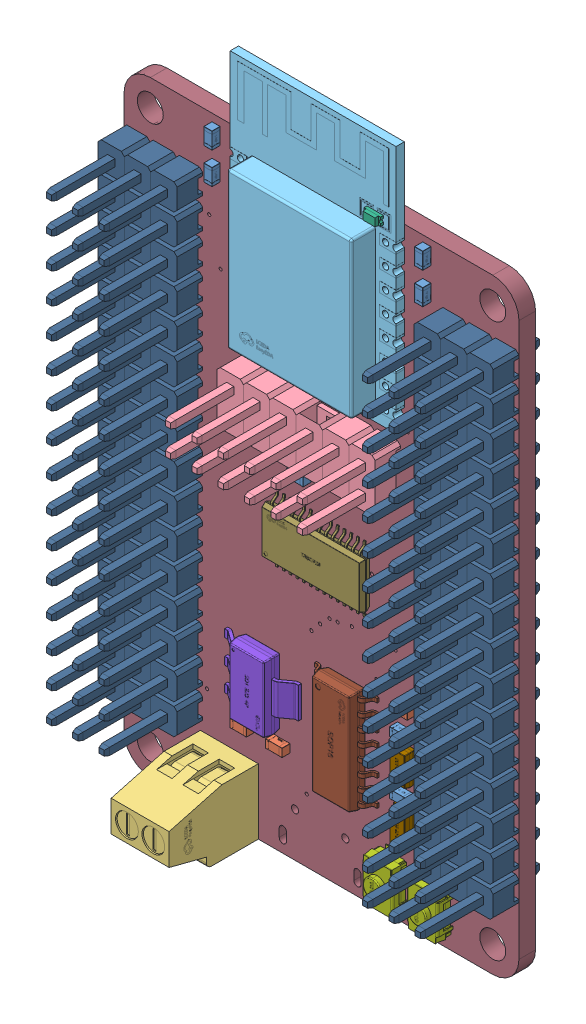
SolidWorks assembly Baize_ServoDriver_esp8266, configuration 默认. Lengths in mm.
Overall size (38.1 65.28 12.15).
165 component instances, 13 part files, 0 mates.
Components (placement in the parent):
- 3D_PCB_PCB_esp8266+pca9685的32路舵机扩展板_2022-08-26_2022-08-26.step-1: 3D_PCB_PCB_esp8266+pca9685的32路舵机扩展板_2022-08-26_2022-08-26.step [默认] at origin size (38.1 65.28 12.15)
  - R8.step-1: R8.step [默认] at (51.4351 43.0531 0) x (1 0 0) z (0 0 -1) size (1.6 0.8 0.8)
    - R0603 NSK.step-1: R0603 NSK.step [默认] at origin size (1.6 0.8 0.8)
      - =_[0_1_1_5].step-1: =_[0_1_1_5].step [默认] at (0 0 0.4) size (1.6 0.8 0.8)
  - R1.step-1: R1.step [默认] at (39.3701 67.0561 1.6) x (0 -1 0) z (0 0 1) size (1.6 0.8 0.8)
    - R0603 NSK.step-1: R0603 NSK.step [默认] at origin size (1.6 0.8 0.8)
      - =_[0_1_1_5].step-1: =_[0_1_1_5].step [默认] at (0 0 0.4) size (1.6 0.8 0.8)
  - R2.step-1: R2.step [默认] at (39.3701 64.0081 1.6) x (0 -1 0) z (0 0 1) size (1.6 0.8 0.8)
    - R0603 NSK.step-1: R0603 NSK.step [默认] at origin size (1.6 0.8 0.8)
      - =_[0_1_1_5].step-1: =_[0_1_1_5].step [默认] at (0 0 0.4) size (1.6 0.8 0.8)
  - R3.step-1: R3.step [默认] at (59.6901 67.1831 1.6) x (0 -1 0) z (0 0 1) size (1.6 0.8 0.8)
    - R0603 NSK.step-1: R0603 NSK.step [默认] at origin size (1.6 0.8 0.8)
      - =_[0_1_1_5].step-1: =_[0_1_1_5].step [默认] at (0 0 0.4) size (1.6 0.8 0.8)
  - R4.step-1: R4.step [默认] at (59.6901 64.1351 1.6) x (0 -1 0) z (0 0 1) size (1.6 0.8 0.8)
    - R0603 NSK.step-1: R0603 NSK.step [默认] at origin size (1.6 0.8 0.8)
      - =_[0_1_1_5].step-1: =_[0_1_1_5].step [默认] at (0 0 0.4) size (1.6 0.8 0.8)
  - R5.step-1: R5.step [默认] at (57.6581 26.2891 1.6) size (1.6 0.8 0.8)
    - R0603 NSK.step-1: R0603 NSK.step [默认] at origin size (1.6 0.8 0.8)
      - =_[0_1_1_5].step-1: =_[0_1_1_5].step [默认] at (0 0 0.4) size (1.6 0.8 0.8)
  - R6.step-1: R6.step [默认] at (57.6581 21.082 1.6) size (1.6 0.8 0.8)
    - R0603 NSK.step-1: R0603 NSK.step [默认] at origin size (1.6 0.8 0.8)
      - =_[0_1_1_5].step-1: =_[0_1_1_5].step [默认] at (0 0 0.4) size (1.6 0.8 0.8)
  - R7.step-1: R7.step [默认] at (47.7521 42.9261 1.6) x (-1 0 0) z (0 0 1) size (1.6 0.8 0.8)
    - R0603 NSK.step-1: R0603 NSK.step [默认] at origin size (1.6 0.8 0.8)
      - =_[0_1_1_5].step-1: =_[0_1_1_5].step [默认] at (0 0 0.4) size (1.6 0.8 0.8)
  - C1.step-1: C1.step [默认] at (42.2911 19.304 1.6) x (-1 0 0) z (0 0 1) size (1.6 0.8 0.8)
    - C0603.step-1: C0603.step [默认] at origin size (1.6 0.8 0.8)
      - =_[0_1_1_16].step-1: =_[0_1_1_16].step [默认] at (0 0 0.4) size (1.6 0.8 0.8)
  - C2.step-1: C2.step [默认] at (45.7201 19.304 1.6) size (1.6 0.8 0.8)
    - C0603.step-1: C0603.step [默认] at origin size (1.6 0.8 0.8)
      - =_[0_1_1_16].step-1: =_[0_1_1_16].step [默认] at (0 0 0.4) size (1.6 0.8 0.8)
  - C3.step-1: C3.step [默认] at (57.7851 28.4481 1.6) size (1.6 0.8 0.8)
    - C0603.step-1: C0603.step [默认] at origin size (1.6 0.8 0.8)
      - =_[0_1_1_16].step-1: =_[0_1_1_16].step [默认] at (0 0 0.4) size (1.6 0.8 0.8)
  - PO.step-1: PO.step [默认] at (40.6401 13.716 1.6) size (5.58 6.3 12.15)
    - CONN-TH_2P-P2.54_JILN_JL308-25402G01.step-1: CONN-TH_2P-P2.54_JILN_JL308-25402G01.step [默认] at origin size (5.58 6.3 12.15)
      - =_[0_1_1_22].step-1: =_[0_1_1_22].step [默认] at (0.05 -0.35 0.05) x (-1 0 0) z (0 0 1) size (5.58 6.3 12.15)
  - GPIO.step-1: GPIO.step [默认] at (49.5301 47.6251 1.6) x (-1 0 0) z (0 0 1) size (15.24 5.09 11.51)
    - HDR-M-2.54_2X6.step-1: HDR-M-2.54_2X6.step [默认] at origin size (15.24 5.09 11.51)
      - COMPOUND.step-1: COMPOUND.step [默认] at origin size (15.24 5.09 11.51)
  - U2.step-1: U2.step [默认] at (49.5301 59.4361 1.6) x (0 -1 0) z (0 0 1) size (24 16.01 3.11)
    - WIFIM-SMD_ESP-12F-ESP8266MOD.step-1: WIFIM-SMD_ESP-12F-ESP8266MOD.step [默认] at origin size (24 16.01 3.11)
      - SOLID.step-1: SOLID.step [默认] at origin size (24 16.01 3.11)
      - COMPOUND-0.step-1: COMPOUND-0.step [默认] at origin size (0.8 1.6 0.6)
  - BOOT.step-1: BOOT.step [默认] at (56.3881 13.462 1.6) x (0 -1 0) z (0 0 1) size (5 3.01 2.4)
    - SW-SMD_L4.0-W2.9-P4.15-EH.step-1: SW-SMD_L4.0-W2.9-P4.15-EH.step [默认] at origin size (5 3.01 2.4)
      - =_[0_1_1_33].step-1: =_[0_1_1_33].step [默认] at (0.009 0 1.5) size (5 3.01 2.4)
  - RST.step-1: RST.step [默认] at (60.7061 13.462 1.6) x (0 -1 0) z (0 0 1) size (5 3.01 2.4)
    - SW-SMD_L4.0-W2.9-P4.15-EH.step-1: SW-SMD_L4.0-W2.9-P4.15-EH.step [默认] at origin size (5 3.01 2.4)
      - =_[0_1_1_33].step-1: =_[0_1_1_33].step [默认] at (0.009 0 1.5) size (5 3.01 2.4)
  - U1.step-1: U1.step [默认] at (43.9421 23.749 1.6) x (-1 0 0) z (0 0 1) size (7.11 6.5 1.75)
    - SOT-223-3_L6.5-W3.4-P2.30-LS7.0-BR.step-1: SOT-223-3_L6.5-W3.4-P2.30-LS7.0-BR.step [默认] at origin size (7.11 6.5 1.75)
      - COMPOUND-1.step-1: COMPOUND-1.step [默认] at origin size (7.11 6.5 1.75)
  - Q1.step-1: Q1.step [默认] at (58.0391 24.003 1.6) x (-1 0 0) z (0 0 1) size (2.81 2.9 1.23)
    - SOT-23-3_L3.0-W1.7-P0.95-LS2.9-BR.step-1: SOT-23-3_L3.0-W1.7-P0.95-LS2.9-BR.step [默认] at origin size (2.81 2.9 1.23)
      - =_[0_1_1_41].step-1: =_[0_1_1_41].step [默认] at (0 0 0.0241) x (-1 0 0) z (0 0 1) size (2.81 2.9 1.23)
  - Q2.step-1: Q2.step [默认] at (58.0391 18.796 1.6) x (-1 0 0) z (0 0 1) size (2.81 2.9 1.23)
    - SOT-23-3_L3.0-W1.7-P0.95-LS2.9-BR.step-1: SOT-23-3_L3.0-W1.7-P0.95-LS2.9-BR.step [默认] at origin size (2.81 2.9 1.23)
      - =_[0_1_1_41].step-1: =_[0_1_1_41].step [默认] at (0 0 0.0241) x (-1 0 0) z (0 0 1) size (2.81 2.9 1.23)
  - S0.step-1: S0.step [默认] at (64.7701 18.415 1.6) size (7.62 2.54 11.5)
    - HDR-M-2.54_1X3.step-1: HDR-M-2.54_1X3.step [默认] at origin size (7.62 2.54 11.5)
      - =_[0_1_1_46].step-1: =_[0_1_1_46].step [默认] at (2.54 0 0) size (7.62 2.54 11.5)
  - S1.step-1: S1.step [默认] at (64.7701 21.336 1.6) size (7.62 2.54 11.5)
    - HDR-M-2.54_1X3.step-1: HDR-M-2.54_1X3.step [默认] at origin size (7.62 2.54 11.5)
      - =_[0_1_1_46].step-1: =_[0_1_1_46].step [默认] at (2.54 0 0) size (7.62 2.54 11.5)
  - S2.step-1: S2.step [默认] at (64.7701 24.257 1.6) size (7.62 2.54 11.5)
    - HDR-M-2.54_1X3.step-1: HDR-M-2.54_1X3.step [默认] at origin size (7.62 2.54 11.5)
      - =_[0_1_1_46].step-1: =_[0_1_1_46].step [默认] at (2.54 0 0) size (7.62 2.54 11.5)
  - S3.step-1: S3.step [默认] at (64.7701 27.1781 1.6) size (7.62 2.54 11.5)
    - HDR-M-2.54_1X3.step-1: HDR-M-2.54_1X3.step [默认] at origin size (7.62 2.54 11.5)
      - =_[0_1_1_46].step-1: =_[0_1_1_46].step [默认] at (2.54 0 0) size (7.62 2.54 11.5)
  - S4.step-1: S4.step [默认] at (64.7701 30.0991 1.6) size (7.62 2.54 11.5)
    - HDR-M-2.54_1X3.step-1: HDR-M-2.54_1X3.step [默认] at origin size (7.62 2.54 11.5)
      - =_[0_1_1_46].step-1: =_[0_1_1_46].step [默认] at (2.54 0 0) size (7.62 2.54 11.5)
  - S5.step-1: S5.step [默认] at (64.7701 33.0201 1.6) size (7.62 2.54 11.5)
    - HDR-M-2.54_1X3.step-1: HDR-M-2.54_1X3.step [默认] at origin size (7.62 2.54 11.5)
      - =_[0_1_1_46].step-1: =_[0_1_1_46].step [默认] at (2.54 0 0) size (7.62 2.54 11.5)
  - S6.step-1: S6.step [默认] at (64.7701 35.9411 1.6) size (7.62 2.54 11.5)
    - HDR-M-2.54_1X3.step-1: HDR-M-2.54_1X3.step [默认] at origin size (7.62 2.54 11.5)
      - =_[0_1_1_46].step-1: =_[0_1_1_46].step [默认] at (2.54 0 0) size (7.62 2.54 11.5)
  - S7.step-1: S7.step [默认] at (64.7701 38.8621 1.6) size (7.62 2.54 11.5)
    - HDR-M-2.54_1X3.step-1: HDR-M-2.54_1X3.step [默认] at origin size (7.62 2.54 11.5)
      - =_[0_1_1_46].step-1: =_[0_1_1_46].step [默认] at (2.54 0 0) size (7.62 2.54 11.5)
  - S8.step-1: S8.step [默认] at (64.7701 41.7831 1.6) size (7.62 2.54 11.5)
    - HDR-M-2.54_1X3.step-1: HDR-M-2.54_1X3.step [默认] at origin size (7.62 2.54 11.5)
      - =_[0_1_1_46].step-1: =_[0_1_1_46].step [默认] at (2.54 0 0) size (7.62 2.54 11.5)
  - S9.step-1: S9.step [默认] at (64.7701 44.7041 1.6) size (7.62 2.54 11.5)
    - HDR-M-2.54_1X3.step-1: HDR-M-2.54_1X3.step [默认] at origin size (7.62 2.54 11.5)
      - =_[0_1_1_46].step-1: =_[0_1_1_46].step [默认] at (2.54 0 0) size (7.62 2.54 11.5)
  - S10.step-1: S10.step [默认] at (64.7701 47.6251 1.6) size (7.62 2.54 11.5)
    - HDR-M-2.54_1X3.step-1: HDR-M-2.54_1X3.step [默认] at origin size (7.62 2.54 11.5)
      - =_[0_1_1_46].step-1: =_[0_1_1_46].step [默认] at (2.54 0 0) size (7.62 2.54 11.5)
  - S11.step-1: S11.step [默认] at (64.7701 50.5461 1.6) size (7.62 2.54 11.5)
    - HDR-M-2.54_1X3.step-1: HDR-M-2.54_1X3.step [默认] at origin size (7.62 2.54 11.5)
      - =_[0_1_1_46].step-1: =_[0_1_1_46].step [默认] at (2.54 0 0) size (7.62 2.54 11.5)
  - S12.step-1: S12.step [默认] at (64.7701 53.4671 1.6) size (7.62 2.54 11.5)
    - HDR-M-2.54_1X3.step-1: HDR-M-2.54_1X3.step [默认] at origin size (7.62 2.54 11.5)
      - =_[0_1_1_46].step-1: =_[0_1_1_46].step [默认] at (2.54 0 0) size (7.62 2.54 11.5)
  - S13.step-1: S13.step [默认] at (64.7701 56.3881 1.6) size (7.62 2.54 11.5)
    - HDR-M-2.54_1X3.step-1: HDR-M-2.54_1X3.step [默认] at origin size (7.62 2.54 11.5)
      - =_[0_1_1_46].step-1: =_[0_1_1_46].step [默认] at (2.54 0 0) size (7.62 2.54 11.5)
  - S14.step-1: S14.step [默认] at (64.7701 59.3091 1.6) size (7.62 2.54 11.5)
    - HDR-M-2.54_1X3.step-1: HDR-M-2.54_1X3.step [默认] at origin size (7.62 2.54 11.5)
      - =_[0_1_1_46].step-1: =_[0_1_1_46].step [默认] at (2.54 0 0) size (7.62 2.54 11.5)
  - S15.step-1: S15.step [默认] at (64.7701 62.2301 1.6) size (7.62 2.54 11.5)
    - HDR-M-2.54_1X3.step-1: HDR-M-2.54_1X3.step [默认] at origin size (7.62 2.54 11.5)
      - =_[0_1_1_46].step-1: =_[0_1_1_46].step [默认] at (2.54 0 0) size (7.62 2.54 11.5)
  - S16.step-1: S16.step [默认] at (34.2901 18.415 1.6) x (-1 0 0) z (0 0 1) size (7.62 2.54 11.5)
    - HDR-M-2.54_1X3.step-1: HDR-M-2.54_1X3.step [默认] at origin size (7.62 2.54 11.5)
      - =_[0_1_1_46].step-1: =_[0_1_1_46].step [默认] at (2.54 0 0) size (7.62 2.54 11.5)
  - S17.step-1: S17.step [默认] at (34.2901 21.336 1.6) x (-1 0 0) z (0 0 1) size (7.62 2.54 11.5)
    - HDR-M-2.54_1X3.step-1: HDR-M-2.54_1X3.step [默认] at origin size (7.62 2.54 11.5)
      - =_[0_1_1_46].step-1: =_[0_1_1_46].step [默认] at (2.54 0 0) size (7.62 2.54 11.5)
  - S18.step-1: S18.step [默认] at (34.2901 24.257 1.6) x (-1 0 0) z (0 0 1) size (7.62 2.54 11.5)
    - HDR-M-2.54_1X3.step-1: HDR-M-2.54_1X3.step [默认] at origin size (7.62 2.54 11.5)
      - =_[0_1_1_46].step-1: =_[0_1_1_46].step [默认] at (2.54 0 0) size (7.62 2.54 11.5)
  - S19.step-1: S19.step [默认] at (34.2901 27.1781 1.6) x (-1 0 0) z (0 0 1) size (7.62 2.54 11.5)
    - HDR-M-2.54_1X3.step-1: HDR-M-2.54_1X3.step [默认] at origin size (7.62 2.54 11.5)
      - =_[0_1_1_46].step-1: =_[0_1_1_46].step [默认] at (2.54 0 0) size (7.62 2.54 11.5)
  - S20.step-1: S20.step [默认] at (34.2901 30.0991 1.6) x (-1 0 0) z (0 0 1) size (7.62 2.54 11.5)
    - HDR-M-2.54_1X3.step-1: HDR-M-2.54_1X3.step [默认] at origin size (7.62 2.54 11.5)
      - =_[0_1_1_46].step-1: =_[0_1_1_46].step [默认] at (2.54 0 0) size (7.62 2.54 11.5)
  - S21.step-1: S21.step [默认] at (34.2901 33.0201 1.6) x (-1 0 0) z (0 0 1) size (7.62 2.54 11.5)
    - HDR-M-2.54_1X3.step-1: HDR-M-2.54_1X3.step [默认] at origin size (7.62 2.54 11.5)
      - =_[0_1_1_46].step-1: =_[0_1_1_46].step [默认] at (2.54 0 0) size (7.62 2.54 11.5)
  - S22.step-1: S22.step [默认] at (34.2901 35.9411 1.6) x (-1 0 0) z (0 0 1) size (7.62 2.54 11.5)
    - HDR-M-2.54_1X3.step-1: HDR-M-2.54_1X3.step [默认] at origin size (7.62 2.54 11.5)
      - =_[0_1_1_46].step-1: =_[0_1_1_46].step [默认] at (2.54 0 0) size (7.62 2.54 11.5)
  - S23.step-1: S23.step [默认] at (34.2901 38.8621 1.6) x (-1 0 0) z (0 0 1) size (7.62 2.54 11.5)
    - HDR-M-2.54_1X3.step-1: HDR-M-2.54_1X3.step [默认] at origin size (7.62 2.54 11.5)
      - =_[0_1_1_46].step-1: =_[0_1_1_46].step [默认] at (2.54 0 0) size (7.62 2.54 11.5)
  - S24.step-1: S24.step [默认] at (34.2901 41.7831 1.6) x (-1 0 0) z (0 0 1) size (7.62 2.54 11.5)
    - HDR-M-2.54_1X3.step-1: HDR-M-2.54_1X3.step [默认] at origin size (7.62 2.54 11.5)
      - =_[0_1_1_46].step-1: =_[0_1_1_46].step [默认] at (2.54 0 0) size (7.62 2.54 11.5)
  - S25.step-1: S25.step [默认] at (34.2901 44.7041 1.6) x (-1 0 0) z (0 0 1) size (7.62 2.54 11.5)
    - HDR-M-2.54_1X3.step-1: HDR-M-2.54_1X3.step [默认] at origin size (7.62 2.54 11.5)
      - =_[0_1_1_46].step-1: =_[0_1_1_46].step [默认] at (2.54 0 0) size (7.62 2.54 11.5)
  - S26.step-1: S26.step [默认] at (34.2901 47.6251 1.6) x (-1 0 0) z (0 0 1) size (7.62 2.54 11.5)
    - HDR-M-2.54_1X3.step-1: HDR-M-2.54_1X3.step [默认] at origin size (7.62 2.54 11.5)
      - =_[0_1_1_46].step-1: =_[0_1_1_46].step [默认] at (2.54 0 0) size (7.62 2.54 11.5)
  - S27.step-1: S27.step [默认] at (34.2901 50.5461 1.6) x (-1 0 0) z (0 0 1) size (7.62 2.54 11.5)
    - HDR-M-2.54_1X3.step-1: HDR-M-2.54_1X3.step [默认] at origin size (7.62 2.54 11.5)
      - =_[0_1_1_46].step-1: =_[0_1_1_46].step [默认] at (2.54 0 0) size (7.62 2.54 11.5)
  - S28.step-1: S28.step [默认] at (34.2901 53.4671 1.6) x (-1 0 0) z (0 0 1) size (7.62 2.54 11.5)
    - HDR-M-2.54_1X3.step-1: HDR-M-2.54_1X3.step [默认] at origin size (7.62 2.54 11.5)
      - =_[0_1_1_46].step-1: =_[0_1_1_46].step [默认] at (2.54 0 0) size (7.62 2.54 11.5)
  - S29.step-1: S29.step [默认] at (34.2901 56.3881 1.6) x (-1 0 0) z (0 0 1) size (7.62 2.54 11.5)
    - HDR-M-2.54_1X3.step-1: HDR-M-2.54_1X3.step [默认] at origin size (7.62 2.54 11.5)
      - =_[0_1_1_46].step-1: =_[0_1_1_46].step [默认] at (2.54 0 0) size (7.62 2.54 11.5)
  - S30.step-1: S30.step [默认] at (34.2901 59.3091 1.6) x (-1 0 0) z (0 0 1) size (7.62 2.54 11.5)
    - HDR-M-2.54_1X3.step-1: HDR-M-2.54_1X3.step [默认] at origin size (7.62 2.54 11.5)
      - =_[0_1_1_46].step-1: =_[0_1_1_46].step [默认] at (2.54 0 0) size (7.62 2.54 11.5)
  - S31.step-1: S31.step [默认] at (34.2901 62.2301 1.6) x (-1 0 0) z (0 0 1) size (7.62 2.54 11.5)
    - HDR-M-2.54_1X3.step-1: HDR-M-2.54_1X3.step [默认] at origin size (7.62 2.54 11.5)
      - =_[0_1_1_46].step-1: =_[0_1_1_46].step [默认] at (2.54 0 0) size (7.62 2.54 11.5)
  - U3.step-1: U3.step [默认] at (52.0701 23.241 1.6) x (0 -1 0) z (0 0 1) size (9.89 6.04 1.68)
    - SOP-16_L10.0-W3.9-P1.27-LS6.0-BL.step-1: SOP-16_L10.0-W3.9-P1.27-LS6.0-BL.step [默认] at origin size (9.89 6.04 1.68)
      - COMPOUND-2.step-1: COMPOUND-2.step [默认] at origin size (9.89 6.04 1.68)
  - U5.step-1: U5.step [默认] at (49.5301 37.0841 0) x (0 1 0) z (0 0 -1) size (6.4 9.69 1.05)
    - TSSOP-28_L9.7-W4.4-P0.65-LS6.4-TL.step-1: TSSOP-28_L9.7-W4.4-P0.65-LS6.4-TL.step [默认] at origin size (6.4 9.69 1.05)
      - COMPOUND-3.step-1: COMPOUND-3.step [默认] at origin size (6.4 9.69 1.05)
  - U4.step-1: U4.step [默认] at (49.5301 37.0841 1.6) x (0 1 0) z (0 0 1) size (6.4 9.69 1.05)
    - TSSOP-28_L9.7-W4.4-P0.65-LS6.4-TL.step-1: TSSOP-28_L9.7-W4.4-P0.65-LS6.4-TL.step [默认] at origin size (6.4 9.69 1.05)
      - COMPOUND-3.step-1: COMPOUND-3.step [默认] at origin size (6.4 9.69 1.05)
  - COMPOUND-4.step-1: COMPOUND-4.step [默认] at origin size (38.07 58.39 1.6)
